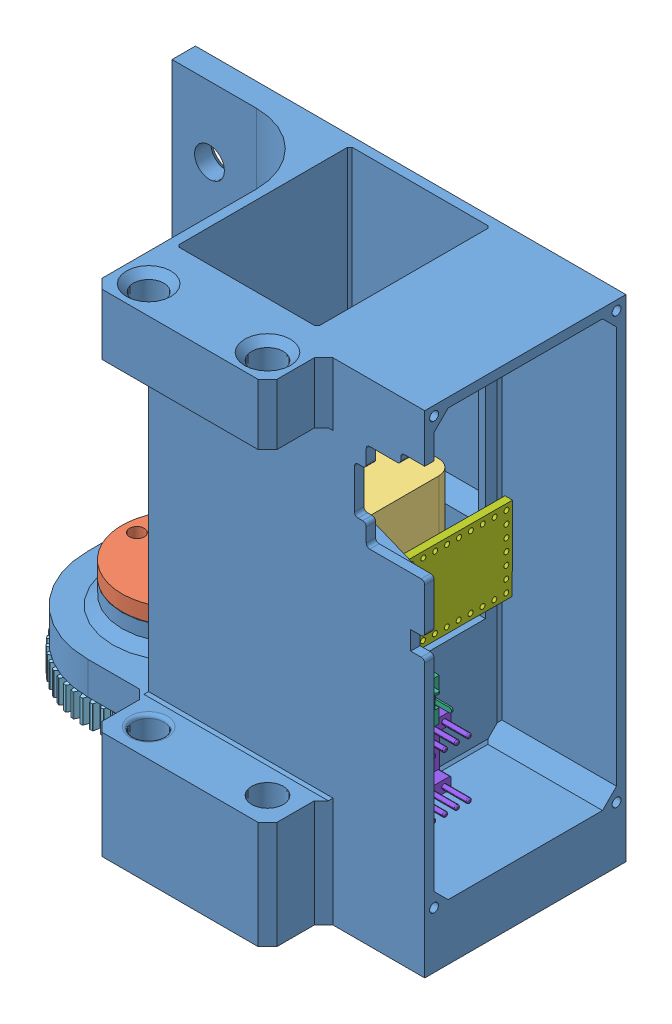
SolidWorks assembly commutator, configuration Default. Lengths in mm.
Overall size (100.87 105 60.87).
8 component instances, 8 part files, 4 mates.
Components (placement in the parent):
- rf_commutator_housing-1: rf_commutator_housing [Default] at origin size (92 105 55)
- Fairview_FMRJ1002_rf_rotary_jpint_female_to_female_flanged-1: Fairview_FMRJ1002_rf_rotary_jpint_female_to_female_flanged [Default] at (0 10.1486 0) x (0 -1 0) z (-0.521112 0 0.853488) size (34.7 25.4 25.4)
- 6627T370_POSITION-CONTROL DC MOTOR-1: 6627T370_POSITION-CONTROL DC MOTOR [6627T37] at (30 13.5246 0) x (0 0 -1) z (0 -1 0) size (28.19 28.19 52.07)
- gear_a-2: gear_a [Default] at (30 -2.3438 0) x (0.979702 0 -0.200458) z (0 -1 0) size (21.12 21.05 5.08)
- gear_b-2: gear_b [Default] at (0 -2.3568 0) x (0.670791 0 0.741646) z (0 -1 0) size (40.88 40.88 13.12)
- CUI_PJ-102A-2: CUI_PJ-102A [Default] at (58.3028 18.2997 9.8994) x (0 -1 0) z (0 0 -1) size (9.4 14.5 14.4)
- Teensy_lc-2: Teensy_lc [Default] at (52.8125 23.9482 17.6843) x (0 1 0) z (-1 0 0) size (17.93 36.98 4.49)
- DRV 8825 With Headers Assem-1: DRV 8825 With Headers Assem [Default] at (67.8565 -6.9624 -1.3078) x (0 0 1) z (-1 0 0) size (21 15 10.9)
Mates (geometry in assembly coordinates):
- Concentric1: concentric anti-aligned: cylinder of rf_commutator_housing-1 through (0 5 0) axis (0 -1 0) radius 7.5; cylinder of Fairview_FMRJ1002_rf_rotary_jpint_female_to_female_flanged-1 through (0 13.4486 0) axis (0 1 0) radius 3.1336
- Concentric2: concentric anti-aligned: cylinder of rf_commutator_housing-1 through (30 5 0) axis (0 -1 0) radius 12.5; cylinder of 6627T370_POSITION-CONTROL DC MOTOR-1 through (30 13.5246 0) axis (0 1 0) radius 10.9982
- Concentric8: concentric anti-aligned: cylinder of Fairview_FMRJ1002_rf_rotary_jpint_female_to_female_flanged-1 through (0 13.4486 0) axis (0 1 0) radius 12.7; cylinder of gear_b-2 through (0 -2.3568 0) axis (0 -1 0) radius 5.425
- Concentric9: concentric aligned: cylinder of 6627T370_POSITION-CONTROL DC MOTOR-1 through (30 -6.5414 0) axis (0 -1 0) radius 2.4994; cylinder of gear_a-2 through (30 -2.3438 0) axis (0 -1 0) radius 2.5
